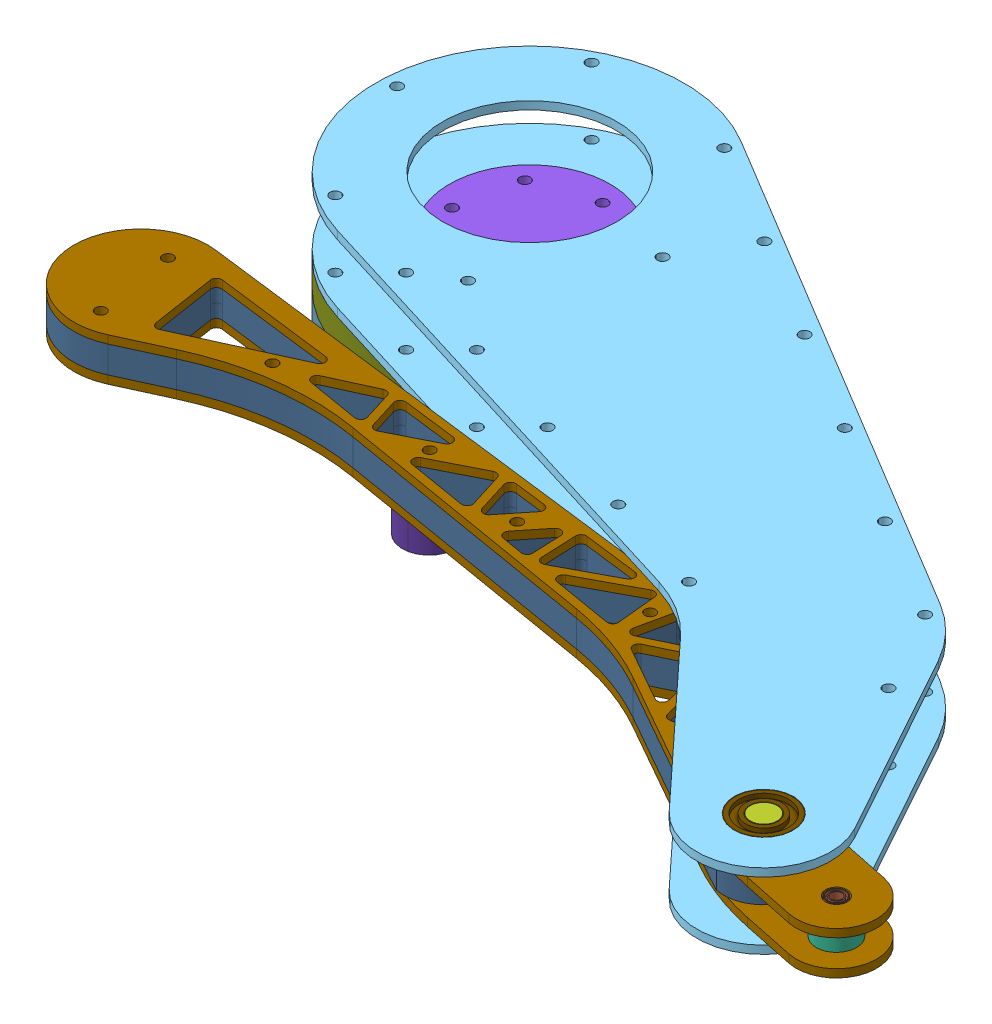
SolidWorks assembly leg, configuration Default. Lengths in mm.
Overall size (407.89 98.4 329.11).
405 component instances, 101 part files, 28 mates.
Components (placement in the parent):
- Cycloidal-1: Cycloidal [Default] at (11.8169 34.4235 32.4982) x (0.945191 0 0.326517) z (-0.326517 0 0.945191) size (162.63 70.39 162.63)
  - motor-X83008S.stp-1: motor-X83008S.stp [Default] at (19.7719 89.7915 55.1095) x (0.817868 0 0.575406) z (0 -1 0) size (114.7 114.7 37.62)
    - base.stp-1: base.stp [Default] at (42.0794 12.0269 46.7342) size (91.6 91.6 15.61)
    - stator.stp-1: stator.stp [Default] at (42.0794 12.0269 33.1342) x (0.08493 -0.996387 0) z (0 0 1) size (83 83 8)
    - coil.stp-1: coil.stp [Default] at (39.5332 41.8984 37.1342) x (0.996387 0.08493 0) z (-0.08493 0.996387 0) size (4.4 10.2 10.5)
    - coil.stp-2: coil.stp [Default] at (34.3848 41.0025 37.1342) x (0.966502 0.256661 0) z (-0.256661 0.966502 0) size (4.4 10.2 10.5)
    - coil.stp-3: coil.stp [Default] at (29.4701 39.2261 37.1342) x (0.90725 0.420593 0) z (-0.420593 0.90725 0) size (4.4 10.2 10.5)
    - coil.stp-4: coil.stp [Default] at (24.9386 36.6233 37.1342) x (0.820431 0.571745 0) z (-0.571745 0.820431 0) size (4.4 10.2 10.5)
    - coil.stp-5: coil.stp [Default] at (20.9279 33.2732 37.1342) x (0.708685 0.705525 0) z (-0.705525 0.708685 0) size (4.4 10.2 10.5)
    - coil.stp-6: coil.stp [Default] at (17.5599 29.2775 37.1342) x (0.575405 0.817869 0) z (-0.817869 0.575405 0) size (4.4 10.2 10.5)
    - coil.stp-7: coil.stp [Default] at (14.9368 24.7576 37.1342) x (0.424642 0.905361 0) z (-0.905361 0.424642 0) size (4.4 10.2 10.5)
    - coil.stp-8: coil.stp [Default] at (13.1385 19.8509 37.1342) x (0.260976 0.965345 0) z (-0.965345 0.260976 0) size (4.4 10.2 10.5)
    - coil.stp-9: coil.stp [Default] at (12.2196 14.7066 37.1342) x (0.089381 0.995998 0) z (-0.995998 0.089381 0) size (4.4 10.2 10.5)
    - coil.stp-10: coil.stp [Default] at (12.2079 9.4807 37.1342) x (-0.08493 0.996387 0) z (-0.996387 -0.08493 0) size (4.4 10.2 10.5)
    - coil.stp-11: coil.stp [Default] at (13.1039 4.3323 37.1342) x (-0.256661 0.966502 0) z (-0.966502 -0.256661 0) size (4.4 10.2 10.5)
    - coil.stp-12: coil.stp [Default] at (14.8802 -0.5824 37.1342) x (-0.420593 0.90725 0) z (-0.90725 -0.420593 0) size (4.4 10.2 10.5)
    - coil.stp-13: coil.stp [Default] at (17.483 -5.1139 37.1342) x (-0.571745 0.820431 0) z (-0.820431 -0.571745 0) size (4.4 10.2 10.5)
    - coil.stp-14: coil.stp [Default] at (20.8332 -9.1246 37.1342) x (-0.705525 0.708685 0) z (-0.708685 -0.705525 0) size (4.4 10.2 10.5)
    - coil.stp-15: coil.stp [Default] at (24.8289 -12.4926 37.1342) x (-0.817869 0.575405 0) z (-0.575405 -0.817869 0) size (4.4 10.2 10.5)
    - coil.stp-16: coil.stp [Default] at (29.3487 -15.1157 37.1342) x (-0.905361 0.424642 0) z (-0.424642 -0.905361 0) size (4.4 10.2 10.5)
    - coil.stp-17: coil.stp [Default] at (34.2554 -16.914 37.1342) x (-0.965345 0.260976 0) z (-0.260976 -0.965345 0) size (4.4 10.2 10.5)
    - coil.stp-18: coil.stp [Default] at (39.3998 -17.8329 37.1342) x (-0.995998 0.089381 0) z (-0.089381 -0.995998 0) size (4.4 10.2 10.5)
    - coil.stp-19: coil.stp [Default] at (44.6256 -17.8446 37.1342) x (-0.996387 -0.08493 0) z (0.08493 -0.996387 0) size (4.4 10.2 10.5)
    - coil.stp-20: coil.stp [Default] at (49.7741 -16.9486 37.1342) x (-0.966502 -0.256661 0) z (0.256661 -0.966502 0) size (4.4 10.2 10.5)
    - coil.stp-21: coil.stp [Default] at (54.6887 -15.1723 37.1342) x (-0.90725 -0.420593 0) z (0.420593 -0.90725 0) size (4.4 10.2 10.5)
    - coil.stp-22: coil.stp [Default] at (59.2202 -12.5695 37.1342) x (-0.820431 -0.571745 0) z (0.571745 -0.820431 0) size (4.4 10.2 10.5)
    - coil.stp-23: coil.stp [Default] at (63.2309 -9.2193 37.1342) x (-0.708685 -0.705525 0) z (0.705525 -0.708685 0) size (4.4 10.2 10.5)
    - coil.stp-24: coil.stp [Default] at (66.599 -5.2236 37.1342) x (-0.575405 -0.817869 0) z (0.817869 -0.575405 0) size (4.4 10.2 10.5)
    - coil.stp-25: coil.stp [Default] at (69.222 -0.7038 37.1342) x (-0.424642 -0.905361 0) z (0.905361 -0.424642 0) size (4.4 10.2 10.5)
    - coil.stp-26: coil.stp [Default] at (71.0203 4.2029 37.1342) x (-0.260976 -0.965345 0) z (0.965345 -0.260976 0) size (4.4 10.2 10.5)
    - coil.stp-27: coil.stp [Default] at (71.9392 9.3473 37.1342) x (-0.089381 -0.995998 0) z (0.995998 -0.089381 0) size (4.4 10.2 10.5)
    - coil.stp-28: coil.stp [Default] at (71.9509 14.5731 37.1342) x (0.08493 -0.996387 0) z (0.996387 0.08493 0) size (4.4 10.2 10.5)
    - coil.stp-29: coil.stp [Default] at (71.055 19.7216 37.1342) x (0.256661 -0.966502 0) z (0.966502 0.256661 0) size (4.4 10.2 10.5)
    - coil.stp-30: coil.stp [Default] at (69.2786 24.6362 37.1342) x (0.420593 -0.90725 0) z (0.90725 0.420593 0) size (4.4 10.2 10.5)
    - coil.stp-31: coil.stp [Default] at (66.6758 29.1677 37.1342) x (0.571745 -0.820431 0) z (0.820431 0.571745 0) size (4.4 10.2 10.5)
    - coil.stp-32: coil.stp [Default] at (63.3257 33.1785 37.1342) x (0.705525 -0.708685 0) z (0.708685 0.705525 0) size (4.4 10.2 10.5)
    - coil.stp-33: coil.stp [Default] at (59.33 36.5465 37.1342) x (0.817869 -0.575405 0) z (0.575405 0.817869 0) size (4.4 10.2 10.5)
    - coil.stp-34: coil.stp [Default] at (54.8101 39.1695 37.1342) x (0.905361 -0.424642 0) z (0.424642 0.905361 0) size (4.4 10.2 10.5)
    - coil.stp-35: coil.stp [Default] at (49.9034 40.9678 37.1342) x (0.965345 -0.260976 0) z (0.260976 0.965345 0) size (4.4 10.2 10.5)
    - coil.stp-36: coil.stp [Default] at (44.759 41.8868 37.1342) x (0.995998 -0.089381 0) z (0.089381 0.995998 0) size (4.4 10.2 10.5)
    - rotor.stp-1: rotor.stp [Default] at (42.0794 12.0269 42.1342) x (-0.293442 0.955977 0) z (0 0 -1) size (91.8 91.8 12)
    - outrunner.stp-1: outrunner.stp [Default] at (42.0794 12.0269 30.1342) x (-0.254711 0.967017 0) z (-0.967017 -0.254711 0) size (91.8 17.01 91.8)
    - screw-mount.stp-1: screw-mount.stp [Default] at (38.1314 27.0157 27.1342) x (1 0 0) z (0 0 -1) size (7 7 6.5)
    - screw-mount.stp-2: screw-mount.stp [Default] at (27.0906 8.0789 27.1342) x (1 0 0) z (0 0 -1) size (7 7 6.5)
    - screw-mount.stp-3: screw-mount.stp [Default] at (57.0682 15.9749 27.1342) x (1 0 0) z (0 0 -1) size (7 7 6.5)
    - screw-mount.stp-4: screw-mount.stp [Default] at (46.0274 -2.9618 27.1342) x (1 0 0) z (0 0 -1) size (7 7 6.5)
    - 6702ZZ-bearing-15x21x4.stp-1: 6702ZZ-bearing-15x21x4.stp [Default] at (42.0794 12.0269 43.7342) x (1 0 0) z (0 -1 0) size (21 4 21)
    - 6702ZZ-bearing-15x21x4.stp-2: 6702ZZ-bearing-15x21x4.stp [Default] at (42.0794 12.0269 35.1342) x (1 0 0) z (0 1 0) size (21 4 21)
    - shaft.stp-1: shaft.stp [Default] at (42.0794 12.0269 20.1342) size (16 16 31.6)
    - fix-screw.stp-1: fix-screw.stp [Default] at (42.0794 12.0269 51.7342) x (1 0 0) z (0 0 -1) size (19.67 18.96 12.02)
  - Base_Plate-1: Base_Plate [Default] at (47.267 69.6573 89.1587) x (-0.64433 0 -0.764747) z (0.764747 0 -0.64433) size (40 7 40)
  - Eccentric_Shaft-1: Eccentric_Shaft [Default] at (62.181 70.3165 95.0179) x (-0.764747 0 0.64433) z (-0.64433 0 -0.764747) size (20 15 17)
    - Eccentric_Shaft_bot-1: Eccentric_Shaft_bot [Default] at (7.6302 6.3409 14.0904) size (17 5 17)
    - Eccentric_Shaft_bot-2: Eccentric_Shaft_bot [Default] at (7.6302 11.3409 14.0904) x (-1 0 0) z (0 0 -1) size (17 5 17)
    - Eccentric_Shaft_top-1: Eccentric_Shaft_top [Default] at (7.6302 16.3409 14.0904) x (-1 0 0) z (0 0 -1) size (17 5 17)
  - Cycloidal_Discs-1: Cycloidal_Discs [Default] at (46.1199 86.6573 90.1252) x (0.999784 0 -0.020763) z (-0.020763 0 -0.999784) size (79.25 5 79.73)
  - Cycloidal_Discs-2: Cycloidal_Discs [Default] at (48.4141 76.6573 88.1922) x (0.979859 0 0.19969) z (-0.19969 0 0.979859) size (79.25 5 79.73)
  - Ring_Pin_Housing-1: Ring_Pin_Housing [Default] at (47.267 76.6573 89.1587) x (0.707107 0 -0.707107) z (0.707107 0 0.707107) size (115 10.6 115)
  - Output_Shaft-1: Output_Shaft [Default] at (47.267 87.2573 89.1587) x (-0.998587 0 -0.053142) z (0.053142 0 -0.998587) size (60 10 60)
  - Cover-1: Cover [Default] at (47.267 87.2573 89.1587) x (0.707107 0 -0.707107) z (0.707107 0 0.707107) size (115 10.4 115)
  - Motor_Cover-2: Motor_Cover [Default] at (47.267 36.0573 89.1587) size (115 33.6 115)
  - radial ball bearing_68_iso-39: radial ball bearing_68_iso [ISO 15 RBB - 1860 - 32,SI,NC,32_68] at (47.267 92.2573 89.1587) x (0 1 0) z (0 0 1) size (10 78 78)
  - radial ball bearing_68_iso-40: radial ball bearing_68_iso [ISO 15 RBB - 1840 - 32,SI,NC,32_68] at (47.267 72.9573 89.1587) x (0 1 0) z (0.001003 0 0.999999) size (7 52 52)
  - Base_plate_2-1: Base_plate_2 [Default] at (47.267 69.6573 89.1587) x (0.707107 0 -0.707107) z (0.707107 0 0.707107) size (115 7 115)
  - m13_bearing-31: m13_bearing [Default] at (-10.7414 95.4081 67.0593) x (0.227678 0 0.973736) z (0.973736 0 -0.227678) size (13 16 13)
    - m6-1: m6 [Default] at (8.4921 2.5508 14.8914) size (6 16 6)
    - radial ball bearing_68_iso-1: radial ball bearing_68_iso [ISO 15 RBB - 286 - 10,SI,NC,10_68] at (8.4921 16.0508 14.8914) x (0 1 0) z (0 0 1) size (5 13 13)
    - radial ball bearing_68_iso-2: radial ball bearing_68_iso [ISO 15 RBB - 286 - 10,SI,NC,10_68] at (8.4921 11.0508 14.8914) x (0 1 0) z (0 0 1) size (5 13 13)
  - m13_bearing-32: m13_bearing [Default] at (-14.1668 95.4081 84.2801) x (0.227678 0 0.973736) z (0.973736 0 -0.227678) size (13 16 13)
    - m6-1: m6 [Default] at (8.4921 2.5508 14.8914) size (6 16 6)
    - radial ball bearing_68_iso-1: radial ball bearing_68_iso [ISO 15 RBB - 286 - 10,SI,NC,10_68] at (8.4921 16.0508 14.8914) x (0 1 0) z (0 0 1) size (5 13 13)
    - radial ball bearing_68_iso-2: radial ball bearing_68_iso [ISO 15 RBB - 286 - 10,SI,NC,10_68] at (8.4921 11.0508 14.8914) x (0 1 0) z (0 0 1) size (5 13 13)
  - m13_bearing-34: m13_bearing [Default] at (13.6125 95.5581 125.8547) x (0.227678 0 0.973736) z (0.973736 0 -0.227678) size (13 16 13)
    - m6-1: m6 [Default] at (8.4921 2.5508 14.8914) size (6 16 6)
    - radial ball bearing_68_iso-1: radial ball bearing_68_iso [ISO 15 RBB - 286 - 10,SI,NC,10_68] at (8.4921 16.0508 14.8914) x (0 1 0) z (0 0 1) size (5 13 13)
    - radial ball bearing_68_iso-2: radial ball bearing_68_iso [ISO 15 RBB - 286 - 10,SI,NC,10_68] at (8.4921 11.0508 14.8914) x (0 1 0) z (0 0 1) size (5 13 13)
  - m13_bearing-35: m13_bearing [Default] at (-0.9866 95.4081 116.0999) x (0.227678 0 0.973736) z (0.973736 0 -0.227678) size (13 16 13)
    - m6-1: m6 [Default] at (8.4921 2.5508 14.8914) size (6 16 6)
    - radial ball bearing_68_iso-1: radial ball bearing_68_iso [ISO 15 RBB - 286 - 10,SI,NC,10_68] at (8.4921 16.0508 14.8914) x (0 1 0) z (0 0 1) size (5 13 13)
    - radial ball bearing_68_iso-2: radial ball bearing_68_iso [ISO 15 RBB - 286 - 10,SI,NC,10_68] at (8.4921 11.0508 14.8914) x (0 1 0) z (0 0 1) size (5 13 13)
  - m13_bearing-36: m13_bearing [Default] at (-10.7414 95.5581 101.5009) x (0.227678 0 0.973736) z (0.973736 0 -0.227678) size (13 16 13)
    - m6-1: m6 [Default] at (8.4921 2.5508 14.8914) size (6 16 6)
    - radial ball bearing_68_iso-1: radial ball bearing_68_iso [ISO 15 RBB - 286 - 10,SI,NC,10_68] at (8.4921 16.0508 14.8914) x (0 1 0) z (0 0 1) size (5 13 13)
    - radial ball bearing_68_iso-2: radial ball bearing_68_iso [ISO 15 RBB - 286 - 10,SI,NC,10_68] at (8.4921 11.0508 14.8914) x (0 1 0) z (0 0 1) size (5 13 13)
  - m13_bearing-1: m13_bearing [Default] at (-0.8801 95.4081 62.5627) x (0.736525 0 0.676411) z (0.676411 0 -0.736525) size (13 16 13)
    - m6-1: m6 [Default] at (8.4921 2.5508 14.8914) size (6 16 6)
    - radial ball bearing_68_iso-1: radial ball bearing_68_iso [ISO 15 RBB - 286 - 10,SI,NC,10_68] at (8.4921 16.0508 14.8914) x (0 1 0) z (0 0 1) size (5 13 13)
    - radial ball bearing_68_iso-2: radial ball bearing_68_iso [ISO 15 RBB - 286 - 10,SI,NC,10_68] at (8.4921 11.0508 14.8914) x (0 1 0) z (0 0 1) size (5 13 13)
  - m13_bearing-2: m13_bearing [Default] at (48.6831 95.4081 124.0939) x (0.120271 0 0.992741) z (0.992741 0 -0.120271) size (13 16 13)
    - m6-1: m6 [Default] at (8.4921 2.5508 14.8914) size (6 16 6)
    - radial ball bearing_68_iso-1: radial ball bearing_68_iso [ISO 15 RBB - 286 - 10,SI,NC,10_68] at (8.4921 16.0508 14.8914) x (0 1 0) z (0 0 1) size (5 13 13)
    - radial ball bearing_68_iso-2: radial ball bearing_68_iso [ISO 15 RBB - 286 - 10,SI,NC,10_68] at (8.4921 11.0508 14.8914) x (0 1 0) z (0 0 1) size (5 13 13)
  - m13_bearing-3: m13_bearing [Default] at (32.7832 95.4081 34.9886) x (-0.046141 0 0.998935) z (0.998935 0 0.046141) size (13 16 13)
    - m6-1: m6 [Default] at (8.4921 2.5508 14.8914) size (6 16 6)
    - radial ball bearing_68_iso-1: radial ball bearing_68_iso [ISO 15 RBB - 286 - 10,SI,NC,10_68] at (8.4921 16.0508 14.8914) x (0 1 0) z (0 0 1) size (5 13 13)
    - radial ball bearing_68_iso-2: radial ball bearing_68_iso [ISO 15 RBB - 286 - 10,SI,NC,10_68] at (8.4921 11.0508 14.8914) x (0 1 0) z (0 0 1) size (5 13 13)
  - m13_bearing-4: m13_bearing [Default] at (77.1902 95.4081 81.0003) x (0.022268 0 0.999752) z (0.999752 0 -0.022268) size (13 16 13)
    - m6-1: m6 [Default] at (8.4921 2.5508 14.8914) size (6 16 6)
    - radial ball bearing_68_iso-1: radial ball bearing_68_iso [ISO 15 RBB - 286 - 10,SI,NC,10_68] at (8.4921 16.0508 14.8914) x (0 1 0) z (0 0 1) size (5 13 13)
    - radial ball bearing_68_iso-2: radial ball bearing_68_iso [ISO 15 RBB - 286 - 10,SI,NC,10_68] at (8.4921 11.0508 14.8914) x (0 1 0) z (0 0 1) size (5 13 13)
  - m13_bearing-5: m13_bearing [Default] at (73.474 95.4081 98.7828) x (0.059133 0 0.99825) z (0.99825 0 -0.059133) size (13 16 13)
    - m6-1: m6 [Default] at (8.4921 2.5508 14.8914) size (6 16 6)
    - radial ball bearing_68_iso-1: radial ball bearing_68_iso [ISO 15 RBB - 286 - 10,SI,NC,10_68] at (8.4921 16.0508 14.8914) x (0 1 0) z (0 0 1) size (5 13 13)
    - radial ball bearing_68_iso-2: radial ball bearing_68_iso [ISO 15 RBB - 286 - 10,SI,NC,10_68] at (8.4921 11.0508 14.8914) x (0 1 0) z (0 0 1) size (5 13 13)
  - m13_bearing-6: m13_bearing [Default] at (12.9248 95.4081 46.7315) x (0.451561 0 0.89224) z (0.89224 0 -0.451561) size (13 16 13)
    - m6-1: m6 [Default] at (8.4921 2.5508 14.8914) size (6 16 6)
    - radial ball bearing_68_iso-1: radial ball bearing_68_iso [ISO 15 RBB - 286 - 10,SI,NC,10_68] at (8.4921 16.0508 14.8914) x (0 1 0) z (0 0 1) size (5 13 13)
    - radial ball bearing_68_iso-2: radial ball bearing_68_iso [ISO 15 RBB - 286 - 10,SI,NC,10_68] at (8.4921 11.0508 14.8914) x (0 1 0) z (0 0 1) size (5 13 13)
  - m13_bearing-7: m13_bearing [Default] at (56.6452 95.4081 32.3406) x (-0.545813 0 0.837907) z (0.837907 0 0.545813) size (13 16 13)
    - m6-1: m6 [Default] at (8.4921 2.5508 14.8914) size (6 16 6)
    - radial ball bearing_68_iso-1: radial ball bearing_68_iso [ISO 15 RBB - 286 - 10,SI,NC,10_68] at (8.4921 16.0508 14.8914) x (0 1 0) z (0 0 1) size (5 13 13)
    - radial ball bearing_68_iso-2: radial ball bearing_68_iso [ISO 15 RBB - 286 - 10,SI,NC,10_68] at (8.4921 11.0508 14.8914) x (0 1 0) z (0 0 1) size (5 13 13)
  - m13_bearing-8: m13_bearing [Default] at (63.0373 95.4081 51.3153) x (0.158553 0 0.98735) z (0.98735 0 -0.158553) size (13 16 13)
    - m6-1: m6 [Default] at (8.4921 2.5508 14.8914) size (6 16 6)
    - radial ball bearing_68_iso-1: radial ball bearing_68_iso [ISO 15 RBB - 286 - 10,SI,NC,10_68] at (8.4921 16.0508 14.8914) x (0 1 0) z (0 0 1) size (5 13 13)
    - radial ball bearing_68_iso-2: radial ball bearing_68_iso [ISO 15 RBB - 286 - 10,SI,NC,10_68] at (8.4921 11.0508 14.8914) x (0 1 0) z (0 0 1) size (5 13 13)
  - m13_bearing-9: m13_bearing [Default] at (83.8577 95.4081 55.5358) x (-0.687134 0 0.72653) z (0.72653 0 0.687134) size (13 16 13)
    - m6-1: m6 [Default] at (8.4921 2.5508 14.8914) size (6 16 6)
    - radial ball bearing_68_iso-1: radial ball bearing_68_iso [ISO 15 RBB - 286 - 10,SI,NC,10_68] at (8.4921 16.0508 14.8914) x (0 1 0) z (0 0 1) size (5 13 13)
    - radial ball bearing_68_iso-2: radial ball bearing_68_iso [ISO 15 RBB - 286 - 10,SI,NC,10_68] at (8.4921 11.0508 14.8914) x (0 1 0) z (0 0 1) size (5 13 13)
  - m13_bearing-11: m13_bearing [Default] at (30.1977 95.4081 135.7424) x (0.57351 0 0.819198) z (0.819198 0 -0.57351) size (13 16 13)
    - m6-1: m6 [Default] at (8.4921 2.5508 14.8914) size (6 16 6)
    - radial ball bearing_68_iso-1: radial ball bearing_68_iso [ISO 15 RBB - 286 - 10,SI,NC,10_68] at (8.4921 16.0508 14.8914) x (0 1 0) z (0 0 1) size (5 13 13)
    - radial ball bearing_68_iso-2: radial ball bearing_68_iso [ISO 15 RBB - 286 - 10,SI,NC,10_68] at (8.4921 11.0508 14.8914) x (0 1 0) z (0 0 1) size (5 13 13)
  - m13_bearing-12: m13_bearing [Default] at (62.8861 95.4081 115.3744) x (0.184178 0 0.982893) z (0.982893 0 -0.184178) size (13 16 13)
    - m6-1: m6 [Default] at (8.4921 2.5508 14.8914) size (6 16 6)
    - radial ball bearing_68_iso-1: radial ball bearing_68_iso [ISO 15 RBB - 286 - 10,SI,NC,10_68] at (8.4921 16.0508 14.8914) x (0 1 0) z (0 0 1) size (5 13 13)
    - radial ball bearing_68_iso-2: radial ball bearing_68_iso [ISO 15 RBB - 286 - 10,SI,NC,10_68] at (8.4921 11.0508 14.8914) x (0 1 0) z (0 0 1) size (5 13 13)
  - socket button head screw_iso-2: socket button head screw_iso [ISO 7380 - M4 x 12 - 12N] at (47.267 67.4573 134.1587) x (0 1 0) z (-0.724148 0 0.689645) size (14.2 7.6 7.6)
  - socket button head screw_iso-3: socket button head screw_iso [ISO 7380 - M4 x 12 - 12N] at (15.4472 67.4573 57.3389) x (0 1 0) z (-0.724148 0 0.689645) size (14.2 7.6 7.6)
  - socket button head screw_iso-4: socket button head screw_iso [ISO 7380 - M4 x 12 - 12N] at (30.0462 67.4573 47.5841) x (0 1 0) z (-0.724148 0 0.689645) size (14.2 7.6 7.6)
  - socket button head screw_iso-5: socket button head screw_iso [ISO 7380 - M4 x 12 - 12N] at (47.267 67.4573 44.1587) x (0 1 0) z (-0.724148 0 0.689645) size (14.2 7.6 7.6)
  - socket button head screw_iso-6: socket button head screw_iso [ISO 7380 - M4 x 12 - 12N] at (64.4877 67.4573 47.5841) x (0 1 0) z (-0.724148 0 0.689645) size (14.2 7.6 7.6)
  - socket button head screw_iso-8: socket button head screw_iso [ISO 7380 - M4 x 12 - 12N] at (88.8416 67.4573 71.9379) x (0 1 0) z (-0.724148 0 0.689645) size (14.2 7.6 7.6)
  - socket button head screw_iso-9: socket button head screw_iso [ISO 7380 - M4 x 12 - 12N] at (92.267 67.4573 89.1587) x (0 1 0) z (-0.724148 0 0.689645) size (14.2 7.6 7.6)
  - socket button head screw_iso-10: socket button head screw_iso [ISO 7380 - M4 x 12 - 12N] at (88.8416 67.4573 106.3794) x (0 1 0) z (-0.724148 0 0.689645) size (14.2 7.6 7.6)
  - socket button head screw_iso-11: socket button head screw_iso [ISO 7380 - M4 x 12 - 12N] at (79.0868 67.4573 120.9785) x (0 1 0) z (-0.724148 0 0.689645) size (14.2 7.6 7.6)
  - M3x35-6: M3x35 [Default] at (9.0832 59.8573 50.9749) size (6 36.2 6)
  - M3x35-7: M3x35 [Default] at (-4.893 59.8573 75.1824) size (6 36.2 6)
  - M3x35-8: M3x35 [Default] at (-4.893 59.8573 103.1349) size (6 36.2 6)
  - M3x35-9: M3x35 [Default] at (9.0832 59.8573 127.3424) size (6 36.2 6)
  - M3x35-10: M3x35 [Default] at (33.2908 59.8573 141.3187) size (6 36.2 6)
  - M3x35-11: M3x35 [Default] at (61.2432 59.8573 141.3187) size (6 36.2 6)
  - M3x35-12: M3x35 [Default] at (85.4508 59.8573 127.3424) size (6 36.2 6)
  - M3x35-13: M3x35 [Default] at (99.427 59.8573 103.1349) size (6 36.2 6)
  - M3x35-14: M3x35 [Default] at (99.427 59.8573 75.1824) size (6 36.2 6)
  - M3x35-15: M3x35 [Default] at (85.4508 59.8573 50.9749) size (6 36.2 6)
  - M3x35-16: M3x35 [Default] at (33.2908 59.8573 36.9987) size (6 36.2 6)
  - M3x35-17: M3x35 [Default] at (61.2432 59.8573 36.9987) size (6 36.2 6)
  - m13_bearing-13: m13_bearing [Default] at (21.9503 95.0081 60.165) x (0 0 1) z (1 0 0) size (13 16 13)
    - m6-1: m6 [Default] at (8.4921 2.5508 14.8914) size (6 16 6)
    - radial ball bearing_68_iso-1: radial ball bearing_68_iso [ISO 15 RBB - 286 - 10,SI,NC,10_68] at (8.4921 16.0508 14.8914) x (0 1 0) z (0 0 1) size (5 13 13)
    - radial ball bearing_68_iso-2: radial ball bearing_68_iso [ISO 15 RBB - 286 - 10,SI,NC,10_68] at (8.4921 11.0508 14.8914) x (0 1 0) z (0 0 1) size (5 13 13)
  - m13_bearing-14: m13_bearing [Default] at (31.351 95.0081 72.3113) x (-0.995553 0 0.094199) z (0.094199 0 0.995553) size (13 16 13)
    - m6-1: m6 [Default] at (8.4921 2.5508 14.8914) size (6 16 6)
    - radial ball bearing_68_iso-1: radial ball bearing_68_iso [ISO 15 RBB - 286 - 10,SI,NC,10_68] at (8.4921 16.0508 14.8914) x (0 1 0) z (0 0 1) size (5 13 13)
    - radial ball bearing_68_iso-2: radial ball bearing_68_iso [ISO 15 RBB - 286 - 10,SI,NC,10_68] at (8.4921 11.0508 14.8914) x (0 1 0) z (0 0 1) size (5 13 13)
  - m13_bearing-15: m13_bearing [Default] at (19.8333 95.0081 99.9459) x (0 0 1) z (1 0 0) size (13 16 13)
    - m6-1: m6 [Default] at (8.4921 2.5508 14.8914) size (6 16 6)
    - radial ball bearing_68_iso-1: radial ball bearing_68_iso [ISO 15 RBB - 286 - 10,SI,NC,10_68] at (8.4921 16.0508 14.8914) x (0 1 0) z (0 0 1) size (5 13 13)
    - radial ball bearing_68_iso-2: radial ball bearing_68_iso [ISO 15 RBB - 286 - 10,SI,NC,10_68] at (8.4921 11.0508 14.8914) x (0 1 0) z (0 0 1) size (5 13 13)
  - m13_bearing-16: m13_bearing [Default] at (60.3496 95.0081 87.0135) x (0.852631 0 -0.522513) z (-0.522513 0 -0.852631) size (13 16 13)
    - m6-1: m6 [Default] at (8.4921 2.5508 14.8914) size (6 16 6)
    - radial ball bearing_68_iso-1: radial ball bearing_68_iso [ISO 15 RBB - 286 - 10,SI,NC,10_68] at (8.4921 16.0508 14.8914) x (0 1 0) z (0 0 1) size (5 13 13)
    - radial ball bearing_68_iso-2: radial ball bearing_68_iso [ISO 15 RBB - 286 - 10,SI,NC,10_68] at (8.4921 11.0508 14.8914) x (0 1 0) z (0 0 1) size (5 13 13)
  - m13_bearing-17: m13_bearing [Default] at (45.2305 95.0081 121.432) x (0.95663 0 0.291306) z (0.291306 0 -0.95663) size (13 16 13)
    - m6-1: m6 [Default] at (8.4921 2.5508 14.8914) size (6 16 6)
    - radial ball bearing_68_iso-1: radial ball bearing_68_iso [ISO 15 RBB - 286 - 10,SI,NC,10_68] at (8.4921 16.0508 14.8914) x (0 1 0) z (0 0 1) size (5 13 13)
    - radial ball bearing_68_iso-2: radial ball bearing_68_iso [ISO 15 RBB - 286 - 10,SI,NC,10_68] at (8.4921 11.0508 14.8914) x (0 1 0) z (0 0 1) size (5 13 13)
  - m13_bearing-18: m13_bearing [Default] at (55.3431 95.0081 81.8889) x (0 0 1) z (1 0 0) size (13 16 13)
    - m6-1: m6 [Default] at (8.4921 2.5508 14.8914) size (6 16 6)
    - radial ball bearing_68_iso-1: radial ball bearing_68_iso [ISO 15 RBB - 286 - 10,SI,NC,10_68] at (8.4921 16.0508 14.8914) x (0 1 0) z (0 0 1) size (5 13 13)
    - radial ball bearing_68_iso-2: radial ball bearing_68_iso [ISO 15 RBB - 286 - 10,SI,NC,10_68] at (8.4921 11.0508 14.8914) x (0 1 0) z (0 0 1) size (5 13 13)
  - M3x4x4.2_brass_insert-1: M3x4x4.2_brass_insert [Default] at (-4.893 93.2573 75.1824) x (0.984609 0 -0.174769) z (0.174769 0 0.984609) size (4 4 4)
  - M3x4x4.2_brass_insert-2: M3x4x4.2_brass_insert [Default] at (9.0832 97.2573 50.9749) x (-0.680278 0 -0.732954) z (-0.732954 0 0.680278) size (4 4 4)
  - M3x4x4.2_brass_insert-3: M3x4x4.2_brass_insert [Default] at (33.2908 97.2573 36.9987) x (-0.509546 0 -0.860444) z (-0.860444 0 0.509546) size (4 4 4)
  - M3x4x4.2_brass_insert-6: M3x4x4.2_brass_insert [Default] at (99.427 97.2573 75.1824) x (-0.680278 0 -0.732954) z (-0.732954 0 0.680278) size (4 4 4)
  - M3x4x4.2_brass_insert-8: M3x4x4.2_brass_insert [Default] at (85.4508 93.2573 127.3424) x (-0.970393 0 0.241533) z (-0.241533 0 -0.970393) size (4 4 4)
  - M3x4x4.2_brass_insert-14: M3x4x4.2_brass_insert [Default] at (61.2432 97.2573 36.9987) x (0.509546 0 0.860444) z (0.860444 0 -0.509546) size (4 4 4)
  - M3x4x4.2_brass_insert-15: M3x4x4.2_brass_insert [Default] at (85.4508 93.2573 50.9749) x (0.897191 0 -0.441644) z (0.441644 0 0.897191) size (4 4 4)
  - M3x4x4.2_brass_insert-16: M3x4x4.2_brass_insert [Default] at (99.427 97.2573 103.1349) x (-0.680278 0 -0.732954) z (-0.732954 0 0.680278) size (4 4 4)
  - M3x4x4.2_brass_insert-17: M3x4x4.2_brass_insert [Default] at (61.2432 97.2573 141.3187) x (0.680278 0 0.732954) z (0.732954 0 -0.680278) size (4 4 4)
  - M3x4x4.2_brass_insert-19: M3x4x4.2_brass_insert [Default] at (33.2908 97.2573 141.3187) x (0.680278 0 0.732954) z (0.732954 0 -0.680278) size (4 4 4)
  - M3x4x4.2_brass_insert-20: M3x4x4.2_brass_insert [Default] at (9.0832 97.2573 127.3424) x (0.680278 0 0.732954) z (0.732954 0 -0.680278) size (4 4 4)
  - M3x4x4.2_brass_insert-21: M3x4x4.2_brass_insert [Default] at (-4.893 97.2573 103.1349) x (0.680278 0 0.732954) z (0.732954 0 -0.680278) size (4 4 4)
  - M4x6x5.5_brass_insert-47: M4x6x5.5_brass_insert [Default] at (5.6924 92.8573 71.9379) x (0.474598 0 0.880203) z (0 1 0) size (5 5 6)
  - M4x6x5.5_brass_insert-48: M4x6x5.5_brass_insert [Default] at (2.267 92.8573 89.1587) x (0.260051 0 0.965595) z (0 1 0) size (5 5 6)
  - M4x6x5.5_brass_insert-49: M4x6x5.5_brass_insert [Default] at (5.6924 87.0073 106.3794) x (-0.745833 0 0.666133) z (0 -1 0) size (5 5 6)
  - M4x6x5.5_brass_insert-50: M4x6x5.5_brass_insert [Default] at (15.4472 86.8573 120.9785) x (-0.745833 0 0.666133) z (0 -1 0) size (5 5 6)
  - M4x6x5.5_brass_insert-51: M4x6x5.5_brass_insert [Default] at (30.0462 87.0073 130.7332) x (0.260051 0 -0.965595) z (0 -1 0) size (5 5 6)
  - M4x6x5.5_brass_insert-1: M4x6x5.5_brass_insert [Default] at (36.8417 86.4573 68.6571) x (-0.745833 0 0.666133) z (0 -1 0) size (5 5 6)
  - M4x6x5.5_brass_insert-4: M4x6x5.5_brass_insert [Default] at (70.2345 92.4573 90.3809) x (0.260051 0 0.965595) z (0 1 0) size (5 5 6)
  - M4x6x5.5_brass_insert-5: M4x6x5.5_brass_insert [Default] at (57.6922 92.4573 109.6602) x (0.260051 0 0.965595) z (0 1 0) size (5 5 6)
  - M4x6x5.5_brass_insert-6: M4x6x5.5_brass_insert [Default] at (34.7247 92.4573 108.438) x (0.260051 0 0.965595) z (0 1 0) size (5 5 6)
  - M4x6x5.5_brass_insert-7: M4x6x5.5_brass_insert [Default] at (24.2995 92.4573 87.9364) x (0.175665 0 0.98445) z (0 1 0) size (5 5 6)
  - M4x6x5.5_brass_insert-8: M4x6x5.5_brass_insert [Default] at (48.4892 97.2573 66.1912) x (0.260051 0 0.965595) z (0 1 0) size (5 5 6)
  - M4x6x5.5_brass_insert-9: M4x6x5.5_brass_insert [Default] at (27.9877 97.2573 76.6164) x (0.260051 0 0.965595) z (0 1 0) size (5 5 6)
  - M4x6x5.5_brass_insert-10: M4x6x5.5_brass_insert [Default] at (26.7654 97.2573 99.5839) x (0.260051 0 0.965595) z (0 1 0) size (5 5 6)
  - M4x6x5.5_brass_insert-11: M4x6x5.5_brass_insert [Default] at (46.0447 97.2573 112.1262) x (0.260051 0 0.965595) z (0 1 0) size (5 5 6)
  - M4x6x5.5_brass_insert-13: M4x6x5.5_brass_insert [Default] at (66.5463 97.2573 101.7009) x (0.260051 0 0.965595) z (0 1 0) size (5 5 6)
  - M4x6x5.5_brass_insert-14: M4x6x5.5_brass_insert [Default] at (67.7686 97.2573 78.7334) x (0.260051 0 0.965595) z (0 1 0) size (5 5 6)
  - M4x6x5.5_brass_insert-15: M4x6x5.5_brass_insert [Default] at (59.8092 92.4573 69.8794) x (0.151918 0 0.988393) z (0 1 0) size (5 5 6)
  - M4x6x5.5_brass_insert-20: M4x6x5.5_brass_insert [Default] at (64.4877 86.8573 130.7332) x (-0.745833 0 0.666133) z (0 -1 0) size (5 5 6)
  - M4x6x5.5_brass_insert-21: M4x6x5.5_brass_insert [Default] at (47.267 86.8573 134.1587) x (-0.745833 0 0.666133) z (0 -1 0) size (5 5 6)
  - M4x6x5.5_brass_insert-22: M4x6x5.5_brass_insert [Default] at (15.4472 86.8573 57.3389) x (0.623293 0 0.781988) z (0 -1 0) size (5 5 6)
  - M4x6x5.5_brass_insert-23: M4x6x5.5_brass_insert [Default] at (30.0462 86.8573 47.5841) x (0.623293 0 0.781988) z (0 -1 0) size (5 5 6)
  - M4x6x5.5_brass_insert-24: M4x6x5.5_brass_insert [Default] at (79.0868 86.8573 120.9785) x (0.541965 0 0.840401) z (0 -1 0) size (5 5 6)
  - M4x6x5.5_brass_insert-25: M4x6x5.5_brass_insert [Default] at (88.8416 86.8573 106.3794) x (-0.745833 0 0.666133) z (0 -1 0) size (5 5 6)
  - M4x6x5.5_brass_insert-26: M4x6x5.5_brass_insert [Default] at (92.267 86.8573 89.1587) x (-0.745833 0 0.666133) z (0 -1 0) size (5 5 6)
  - M4x6x5.5_brass_insert-27: M4x6x5.5_brass_insert [Default] at (88.8416 86.8573 71.9379) x (-0.745833 0 0.666133) z (0 -1 0) size (5 5 6)
  - M4x6x5.5_brass_insert-28: M4x6x5.5_brass_insert [Default] at (79.0868 92.8573 57.3389) x (0.260051 0 0.965595) z (0 1 0) size (5 5 6)
  - M4x6x5.5_brass_insert-29: M4x6x5.5_brass_insert [Default] at (64.4877 86.8573 47.5841) x (-0.142939 0 0.989731) z (0 -1 0) size (5 5 6)
  - M4x6x5.5_brass_insert-31: M4x6x5.5_brass_insert [Default] at (47.267 86.8573 44.1587) x (-0.220341 0 0.975423) z (0 -1 0) size (5 5 6)
  - M4x6x5.5_brass_insert-34: M4x6x5.5_brass_insert [Default] at (1.8007 97.2573 62.9087) x (0.260051 0 0.965595) z (0 1 0) size (5 5 6)
  - M4x6x5.5_brass_insert-35: M4x6x5.5_brass_insert [Default] at (-5.233 97.2573 89.1587) x (0.260051 0 0.965595) z (0 1 0) size (5 5 6)
  - M4x6x5.5_brass_insert-36: M4x6x5.5_brass_insert [Default] at (1.8007 97.2573 115.4087) x (0.260051 0 0.965595) z (0 1 0) size (5 5 6)
  - M4x6x5.5_brass_insert-37: M4x6x5.5_brass_insert [Default] at (21.017 97.2573 134.625) x (0.260051 0 0.965595) z (0 1 0) size (5 5 6)
  - M4x6x5.5_brass_insert-38: M4x6x5.5_brass_insert [Default] at (47.267 97.2573 141.6587) x (0.260051 0 0.965595) z (0 1 0) size (5 5 6)
  - M4x6x5.5_brass_insert-39: M4x6x5.5_brass_insert [Default] at (73.517 97.2573 134.625) x (0.260051 0 0.965595) z (0 1 0) size (5 5 6)
  - M4x6x5.5_brass_insert-40: M4x6x5.5_brass_insert [Default] at (92.7333 97.2573 115.4087) x (0.260051 0 0.965595) z (0 1 0) size (5 5 6)
  - M4x6x5.5_brass_insert-41: M4x6x5.5_brass_insert [Default] at (99.767 97.2573 89.1587) x (0.260051 0 0.965595) z (0 1 0) size (5 5 6)
  - M4x6x5.5_brass_insert-42: M4x6x5.5_brass_insert [Default] at (92.7333 97.2573 62.9087) x (0.260051 0 0.965595) z (0 1 0) size (5 5 6)
  - M4x6x5.5_brass_insert-43: M4x6x5.5_brass_insert [Default] at (73.517 97.2573 43.6923) x (0.260051 0 0.965595) z (0 1 0) size (5 5 6)
  - M4x6x5.5_brass_insert-44: M4x6x5.5_brass_insert [Default] at (47.267 97.2573 36.6587) x (0.260051 0 0.965595) z (0 1 0) size (5 5 6)
  - M4x6x5.5_brass_insert-45: M4x6x5.5_brass_insert [Default] at (21.017 97.2573 43.6923) x (0.260051 0 0.965595) z (0 1 0) size (5 5 6)
  - pan cross head_am-1: pan cross head_am [B18.6.7M - M3 x 0.5 x 20 Type I Cross Recessed PHMS --20N] at (44.6897 92.5573 86.0997) x (0 -1 0) z (0.748822 0 0.662771) size (22.37 5.6 5.6)
  - pan cross head_am-3: pan cross head_am [B18.6.7M - M3 x 0.5 x 20 Type I Cross Recessed PHMS --20N] at (49.8443 92.5573 92.2177) x (0 -1 0) z (0.940321 0 0.340288) size (22.37 5.6 5.6)
  - M3x4x4.2_brass_insert-22: M3x4x4.2_brass_insert [Default] at (44.6897 69.6573 86.0997) x (0.984609 0 -0.174769) z (0.174769 0 0.984609) size (4 4 4)
  - M3x4x4.2_brass_insert-23: M3x4x4.2_brass_insert [Default] at (49.8443 69.6573 92.2177) x (0.984609 0 -0.174769) z (0.174769 0 0.984609) size (4 4 4)
  - pan cross head_am-4: pan cross head_am [B18.6.7M - M3 x 0.5 x 10 Type I Cross Recessed PHMS --10N] at (57.2541 77.5573 101.0123) x (0 -1 0) z (0 0 1) size (12.37 5.6 5.6)
  - pan cross head_am-5: pan cross head_am [B18.6.7M - M3 x 0.5 x 10 Type I Cross Recessed PHMS --10N] at (37.2799 77.5573 77.3051) x (0 -1 0) z (0 0 1) size (12.37 5.6 5.6)
  - pan cross head_am-6: pan cross head_am [B18.6.7M - M3 x 0.5 x 10 Type I Cross Recessed PHMS --10N] at (59.1206 77.5573 79.1715) x (0 -1 0) z (0 0 1) size (12.37 5.6 5.6)
  - pan cross head_am-7: pan cross head_am [B18.6.7M - M3 x 0.5 x 10 Type I Cross Recessed PHMS --10N] at (35.4134 77.5573 99.1458) x (0 -1 0) z (0 0 1) size (12.37 5.6 5.6)
  - radial ball bearing_68_iso-44: radial ball bearing_68_iso [ISO 15 RBB - 1715 - 26,SI,NC,26_68] at (46.1199 84.6573 90.1252) x (0 1 0) z (-0.714953 0 -0.699173) size (4 21 21)
  - radial ball bearing_68_iso-45: radial ball bearing_68_iso [ISO 15 RBB - 1715 - 26,SI,NC,26_68] at (47.267 89.6573 89.1587) x (0 1 0) z (0.999483 0 -0.032163) size (4 21 21)
  - radial ball bearing_68_iso-46: radial ball bearing_68_iso [ISO 15 RBB - 1715 - 26,SI,NC,26_68] at (48.4141 79.6573 88.1922) x (0 1 0) z (0 0 1) size (4 21 21)
  - socket button head screw_iso-37: socket button head screw_iso [ISO 7380 - M4 x 12 - 12N] at (79.0868 67.4573 57.3389) x (0 1 0) z (-0.709975 0 0.704227) size (14.2 7.6 7.6)
  - socket button head screw_iso-38: socket button head screw_iso [ISO 7380 - M4 x 12 - 12N] at (64.4877 67.4573 130.7332) x (0 1 0) z (-0.724148 0 0.689645) size (14.2 7.6 7.6)
  - foc-motor-controller.step-1: foc-motor-controller.step [Default] at (47.267 33.6573 89.1587) x (0.707107 0 0.707107) z (0 -1 0) size (57.23 50 8.13)
    - RTA0040B.step-1: RTA0040B.step [Default] at (12.5014 -1.6986 1.595) x (-0.707107 -0.707107 0) z (0 0 1) size (6 6 1)
      - FRAME.step-1: FRAME.step [Default] x (1 0 0) z (0 -1 0) size (6 0.2 6)
        - SOLID.step-1: SOLID.step [Default] at origin size (0.4 0.2 0.22)
        - SOLID-0.step-1: SOLID-0.step [Default] at origin size (0.4 0.2 0.22)
        - SOLID-1.step-1: SOLID-1.step [Default] at origin size (0.4 0.2 0.22)
